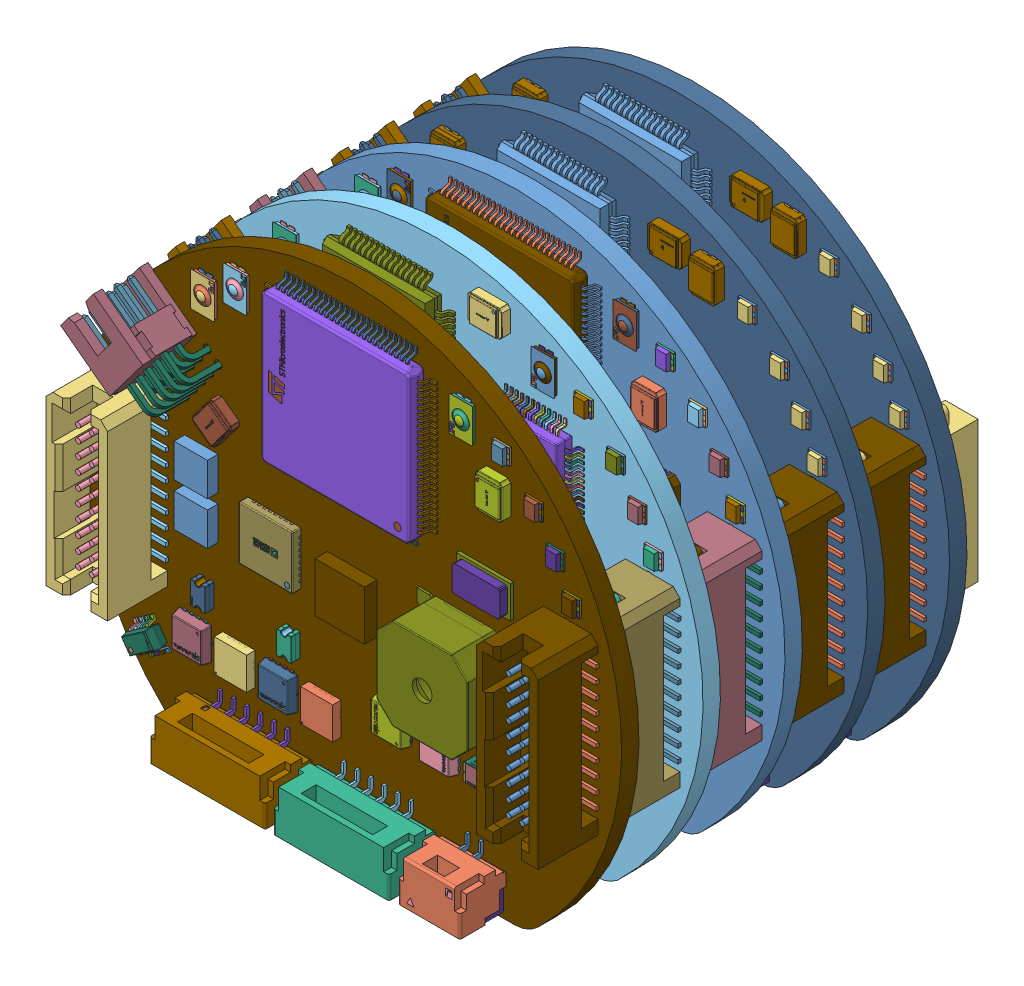
SolidWorks assembly ASSY_HYDRA_MASTER, configuration Default. Lengths in mm.
Overall size (50.15 44.15 42.22).
698 component instances, 436 part files, 12 mates.
Components (placement in the parent):
- HYDRA_V4_NAV-1: HYDRA_V4_NAV [Default] at origin size (50 44 11.77)
  - Open CASCADE STEP translator 7.5 734-1: Open CASCADE STEP translator 7.5 734 [Default] at origin size (50 44 1.75)
  - Open CASCADE STEP translator 7.5 766-1: Open CASCADE STEP translator 7.5 766 [Default] at origin size (2.53 3.23 1.01)
  - Open CASCADE STEP translator 7.5 767-1: Open CASCADE STEP translator 7.5 767 [Default] at origin size (2.5 3.2 0)
  - Open CASCADE STEP translator 7.5 769-1: Open CASCADE STEP translator 7.5 769 [Default] at origin size (0.26 1.24 0)
  - Open CASCADE STEP translator 7.5 770-1: Open CASCADE STEP translator 7.5 770 [Default] at origin size (2.9 1.6 1.31)
  - Open CASCADE STEP translator 7.5 771-1: Open CASCADE STEP translator 7.5 771 [Default] at origin size (0.3 0.6 0.86)
  - Open CASCADE STEP translator 7.5 772-1: Open CASCADE STEP translator 7.5 772 [Default] at origin size (0.3 0.6 0.86)
  - Open CASCADE STEP translator 7.5 773-1: Open CASCADE STEP translator 7.5 773 [Default] at origin size (0.3 0.6 0.86)
  - Open CASCADE STEP translator 7.5 774-1: Open CASCADE STEP translator 7.5 774 [Default] at origin size (0.3 0.6 0.86)
  - Open CASCADE STEP translator 7.5 775-1: Open CASCADE STEP translator 7.5 775 [Default] at origin size (0.4 0.4 0.01)
  - Open CASCADE STEP translator 7.5 776-1: Open CASCADE STEP translator 7.5 776 [Default] at origin size (0.29 1.22 0.01)
  - Open CASCADE STEP translator 7.5 777-1: Open CASCADE STEP translator 7.5 777 [Default] at origin size (0.3 0.6 0.86)
  - Open CASCADE STEP translator 7.5 778-1: Open CASCADE STEP translator 7.5 778 [Default] at origin size (0.3 0.6 0.86)
  - Open CASCADE STEP translator 7.5 779-1: Open CASCADE STEP translator 7.5 779 [Default] at origin size (0.3 0.6 0.86)
  - Open CASCADE STEP translator 7.5 780-1: Open CASCADE STEP translator 7.5 780 [Default] at origin size (0.3 0.6 0.86)
  - Open CASCADE STEP translator 7.5 781-1: Open CASCADE STEP translator 7.5 781 [Default] at origin size (3.25 2.93 1.32)
  - Open CASCADE STEP translator 7.5 782-1: Open CASCADE STEP translator 7.5 782 [Default] at origin size (0.59 0.66 0.86)
  - Open CASCADE STEP translator 7.5 783-1: Open CASCADE STEP translator 7.5 783 [Default] at origin size (0.59 0.66 0.86)
  - Open CASCADE STEP translator 7.5 784-1: Open CASCADE STEP translator 7.5 784 [Default] at origin size (0.59 0.66 0.86)
  - Open CASCADE STEP translator 7.5 785-1: Open CASCADE STEP translator 7.5 785 [Default] at origin size (0.59 0.66 0.86)
  - Open CASCADE STEP translator 7.5 786-1: Open CASCADE STEP translator 7.5 786 [Default] at origin size (0.4 0.4 0.01)
  - Open CASCADE STEP translator 7.5 787-1: Open CASCADE STEP translator 7.5 787 [Default] at origin size (0.65 1.09 0.01)
  - Open CASCADE STEP translator 7.5 788-1: Open CASCADE STEP translator 7.5 788 [Default] at origin size (0.59 0.66 0.86)
  - Open CASCADE STEP translator 7.5 789-1: Open CASCADE STEP translator 7.5 789 [Default] at origin size (0.59 0.66 0.86)
  - Open CASCADE STEP translator 7.5 790-1: Open CASCADE STEP translator 7.5 790 [Default] at origin size (0.59 0.66 0.86)
  - Open CASCADE STEP translator 7.5 791-1: Open CASCADE STEP translator 7.5 791 [Default] at origin size (0.59 0.66 0.86)
  - Open CASCADE STEP translator 7.5 833-1: Open CASCADE STEP translator 7.5 833 [Default] at origin size (0.2 2.2 2.05)
  - Open CASCADE STEP translator 7.5 834-1: Open CASCADE STEP translator 7.5 834 [Default] at origin size (0.2 2.2 2.05)
  - Open CASCADE STEP translator 7.5 835-1: Open CASCADE STEP translator 7.5 835 [Default] at origin size (1.45 1.3 1.05)
  - Open CASCADE STEP translator 7.5 836-1: Open CASCADE STEP translator 7.5 836 [Default] at origin size (5.75 4.05 4.25)
  - Open CASCADE STEP translator 7.5 837-1: Open CASCADE STEP translator 7.5 837 [Default] at origin size (1.45 2.03 0.46)
  - Open CASCADE STEP translator 7.5 838-1: Open CASCADE STEP translator 7.5 838 [Default] at origin size (4.2 3.06 0.01)
  - Open CASCADE STEP translator 7.5 839-1: Open CASCADE STEP translator 7.5 839 [Default] at origin size (14.1 15.2 1.88)
  - Open CASCADE STEP translator 7.5 863-1: Open CASCADE STEP translator 7.5 863 [Default] at origin size (4.1 4.1 0.98)
  - Open CASCADE STEP translator 7.5 864-1: Open CASCADE STEP translator 7.5 864 [Default] at origin size (4.53 6.4 0.96)
  - Open CASCADE STEP translator 7.5 865-1: Open CASCADE STEP translator 7.5 865 [Default] at origin size (6.2 6.4 0.64)
  - Open CASCADE STEP translator 7.5 866-1: Open CASCADE STEP translator 7.5 866 [Default] at origin size (5.96 5.96 2.39)
  - Open CASCADE STEP translator 7.5 867-1: Open CASCADE STEP translator 7.5 867 [Default] at origin size (4.4 4.4 0.72)
  - Open CASCADE STEP translator 7.5 868-1: Open CASCADE STEP translator 7.5 868 [Default] at origin size (6.1 6 0)
  - Open CASCADE STEP translator 7.5 869-1: Open CASCADE STEP translator 7.5 869 [Default] at origin size (0.75 2.66 0)
  - Open CASCADE STEP translator 7.5 870-1: Open CASCADE STEP translator 7.5 870 [Default] at origin size (3.1 3.1 1)
  - Open CASCADE STEP translator 7.5 871-1: Open CASCADE STEP translator 7.5 871 [Default] at origin size (3 2.5 0.81)
  - Open CASCADE STEP translator 7.5 1038-1: Open CASCADE STEP translator 7.5 1038 [Default] at origin size (1.6 1.5 0.2)
  - Open CASCADE STEP translator 7.5 1039-1: Open CASCADE STEP translator 7.5 1039 [Default] at origin size (1.6 1.4 0.19)
  - Open CASCADE STEP translator 7.5 1040-1: Open CASCADE STEP translator 7.5 1040 [Default] at origin size (1.1 1.5 0.36)
  - Open CASCADE STEP translator 7.5 1113-1: Open CASCADE STEP translator 7.5 1113 [Default] at origin size (4.71 4.67 1.1)
  - Open CASCADE STEP translator 7.5 1118-1: Open CASCADE STEP translator 7.5 1118 [Default] at origin size (1.6 1.5 0.2)
  - Open CASCADE STEP translator 7.5 1119-1: Open CASCADE STEP translator 7.5 1119 [Default] at origin size (1.6 1.4 0.19)
  - Open CASCADE STEP translator 7.5 1120-1: Open CASCADE STEP translator 7.5 1120 [Default] at origin size (1.1 1.5 0.36)
  - Open CASCADE STEP translator 7.5 1124-1: Open CASCADE STEP translator 7.5 1124 [Default] at origin size (10.4 9.7 2.7)
  - Open CASCADE STEP translator 7.5 1125-1: Open CASCADE STEP translator 7.5 1125 [Default] at origin size (5 3 0.3)
  - Open CASCADE STEP translator 7.5 1126-1: Open CASCADE STEP translator 7.5 1126 [Default] at origin size (4.46 2.46 0.7)
  - Open CASCADE STEP translator 7.5 1127-1: Open CASCADE STEP translator 7.5 1127 [Default] at origin size (4.6 4.6 1.15)
  - Open CASCADE STEP translator 7.5 1128-1: Open CASCADE STEP translator 7.5 1128 [Default] at origin size (14 14 1.52)
  - Open CASCADE STEP translator 7.5 1129-1: Open CASCADE STEP translator 7.5 1129 [Default] at origin size (16 12.22 0.95)
  - Open CASCADE STEP translator 7.5 1130-1: Open CASCADE STEP translator 7.5 1130 [Default] at origin size (12.22 16 0.95)
  - Open CASCADE STEP translator 7.5 1131-1: Open CASCADE STEP translator 7.5 1131 [Default] at origin size (12.33 12.46 0.1)
  - Open CASCADE STEP translator 7.5 1132-1: Open CASCADE STEP translator 7.5 1132 [Default] at origin size (1.3 3.5 0.06)
  - Open CASCADE STEP translator 7.5 1133-1: Open CASCADE STEP translator 7.5 1133 [Default] at origin size (2 3 0.57)
  - Open CASCADE STEP translator 7.5 1134-1: Open CASCADE STEP translator 7.5 1134 [Default] at origin size (2.2 3.2 0.32)
  - Open CASCADE STEP translator 7.5 1135-1: Open CASCADE STEP translator 7.5 1135 [Default] at origin size (0.46 0.93 0.01)
  - Open CASCADE STEP translator 7.5 1136-1: Open CASCADE STEP translator 7.5 1136 [Default] at origin size (1.3 3.5 0.06)
  - Open CASCADE STEP translator 7.5 1137-1: Open CASCADE STEP translator 7.5 1137 [Default] at origin size (2 3 0.57)
  - Open CASCADE STEP translator 7.5 1138-1: Open CASCADE STEP translator 7.5 1138 [Default] at origin size (2.2 3.2 0.32)
  - Open CASCADE STEP translator 7.5 1139-1: Open CASCADE STEP translator 7.5 1139 [Default] at origin size (0.46 0.93 0.01)
  - Open CASCADE STEP translator 7.5 1209-1: Open CASCADE STEP translator 7.5 1209 [Default] at origin size (2.6 2.6 0.35)
  - Open CASCADE STEP translator 7.5 1210-1: Open CASCADE STEP translator 7.5 1210 [Default] at origin size (7.98 7.97 5.08)
  - Open CASCADE STEP translator 7.5 1211-1: Open CASCADE STEP translator 7.5 1211 [Default] at origin size (6.65 6.86 1.68)
  - Open CASCADE STEP translator 7.5 1212-1: Open CASCADE STEP translator 7.5 1212 [Default] at origin size (6.1 6.49 5.65)
  - Open CASCADE STEP translator 7.5 1213-1: Open CASCADE STEP translator 7.5 1213 [Default] at origin size (11.95 7.6 2.76)
  - Open CASCADE STEP translator 7.5 1214-1: Open CASCADE STEP translator 7.5 1214 [Default] at origin size (1.9 6.7 2.22)
  - Open CASCADE STEP translator 7.5 1215-1: Open CASCADE STEP translator 7.5 1215 [Default] at origin size (6.4 5 1.77)
  - Open CASCADE STEP translator 7.5 1216-1: Open CASCADE STEP translator 7.5 1216 [Default] at origin size (4.77 4.35 0.13)
  - Open CASCADE STEP translator 7.5 1217-1: Open CASCADE STEP translator 7.5 1217 [Default] at origin size (1.9 6.7 2.22)
  - Open CASCADE STEP translator 7.5 1293-1: Open CASCADE STEP translator 7.5 1293 [Default] at origin size (1.6 1.5 0.2)
  - Open CASCADE STEP translator 7.5 1294-1: Open CASCADE STEP translator 7.5 1294 [Default] at origin size (1.6 1.4 0.19)
  - Open CASCADE STEP translator 7.5 1295-1: Open CASCADE STEP translator 7.5 1295 [Default] at origin size (1.1 1.5 0.36)
  - Open CASCADE STEP translator 7.5 1296-1: Open CASCADE STEP translator 7.5 1296 [Default] at origin size (1.6 1.5 0.2)
  - Open CASCADE STEP translator 7.5 1297-1: Open CASCADE STEP translator 7.5 1297 [Default] at origin size (1.6 1.4 0.19)
  - Open CASCADE STEP translator 7.5 1298-1: Open CASCADE STEP translator 7.5 1298 [Default] at origin size (1.1 1.5 0.36)
  - Open CASCADE STEP translator 7.5 1299-1: Open CASCADE STEP translator 7.5 1299 [Default] at origin size (1.3 3.5 0.06)
  - Open CASCADE STEP translator 7.5 1300-1: Open CASCADE STEP translator 7.5 1300 [Default] at origin size (2 3 0.57)
  - Open CASCADE STEP translator 7.5 1301-1: Open CASCADE STEP translator 7.5 1301 [Default] at origin size (2.2 3.2 0.32)
  - Open CASCADE STEP translator 7.5 1302-1: Open CASCADE STEP translator 7.5 1302 [Default] at origin size (0.46 0.93 0.01)
  - Open CASCADE STEP translator 7.5 1303-1: Open CASCADE STEP translator 7.5 1303 [Default] at origin size (5.72 15.88 6.73)
  - Open CASCADE STEP translator 7.5 1304-1: Open CASCADE STEP translator 7.5 1304 [Default] at origin size (1.78 12.7 4.01)
  - Open CASCADE STEP translator 7.5 1305-1: Open CASCADE STEP translator 7.5 1305 [Default] at origin size (5.84 12.7 0.83)
  - Open CASCADE STEP translator 7.5 1306-1: Open CASCADE STEP translator 7.5 1306 [Default] at origin size (5.72 15.88 6.73)
  - Open CASCADE STEP translator 7.5 1307-1: Open CASCADE STEP translator 7.5 1307 [Default] at origin size (1.78 12.7 4.01)
  - Open CASCADE STEP translator 7.5 1308-1: Open CASCADE STEP translator 7.5 1308 [Default] at origin size (5.84 12.7 0.83)
  - Open CASCADE STEP translator 7.5 1309-1: Open CASCADE STEP translator 7.5 1309 [Default] at origin size (3.68 15.88 5.84)
  - Open CASCADE STEP translator 7.5 1310-1: Open CASCADE STEP translator 7.5 1310 [Default] at origin size (4.09 12.7 1.18)
  - Open CASCADE STEP translator 7.5 1311-1: Open CASCADE STEP translator 7.5 1311 [Default] at origin size (3.68 15.88 5.84)
  - Open CASCADE STEP translator 7.5 1312-1: Open CASCADE STEP translator 7.5 1312 [Default] at origin size (4.09 12.7 1.18)
- HYDRA_V4_LINK_V2-1: HYDRA_V4_LINK_V2 [Default] at (-0.0024 -0.0016 7.6116) size (50 44 11.77)
  - Open CASCADE STEP translator 7.5 1-1: Open CASCADE STEP translator 7.5 1 [Default] at origin size (50 44 1.61)
  - Open CASCADE STEP translator 7.5 16-1: Open CASCADE STEP translator 7.5 16 [Default] at origin size (13.25 4.05 4.25)
  - Open CASCADE STEP translator 7.5 17-1: Open CASCADE STEP translator 7.5 17 [Default] at origin size (0.2 4.65 2.09)
  - Open CASCADE STEP translator 7.5 18-1: Open CASCADE STEP translator 7.5 18 [Default] at origin size (0.2 4.65 2.09)
  - Open CASCADE STEP translator 7.5 19-1: Open CASCADE STEP translator 7.5 19 [Default] at origin size (0.2 4.65 2.09)
  - Open CASCADE STEP translator 7.5 20-1: Open CASCADE STEP translator 7.5 20 [Default] at origin size (0.2 4.65 2.09)
  - Open CASCADE STEP translator 7.5 21-1: Open CASCADE STEP translator 7.5 21 [Default] at origin size (0.2 4.65 2.09)
  - Open CASCADE STEP translator 7.5 22-1: Open CASCADE STEP translator 7.5 22 [Default] at origin size (0.2 4.65 2.09)
  - Open CASCADE STEP translator 7.5 23-1: Open CASCADE STEP translator 7.5 23 [Default] at origin size (0.2 4.65 2.09)
  - Open CASCADE STEP translator 7.5 24-1: Open CASCADE STEP translator 7.5 24 [Default] at origin size (0.2 4.65 2.09)
  - Open CASCADE STEP translator 7.5 86-1: Open CASCADE STEP translator 7.5 86 [Default] at origin size (2.15 1.35 0.85)
  - Open CASCADE STEP translator 7.5 87-1: Open CASCADE STEP translator 7.5 87 [Default] at origin size (2.15 1.35 0.85)
  - Open CASCADE STEP translator 7.5 88-1: Open CASCADE STEP translator 7.5 88 [Default] at origin size (1.21 0.73 0.02)
  - Open CASCADE STEP translator 7.5 89-1: Open CASCADE STEP translator 7.5 89 [Default] at origin size (3.23 2.53 1.01)
  - Open CASCADE STEP translator 7.5 90-1: Open CASCADE STEP translator 7.5 90 [Default] at origin size (3.2 2.5 0)
  - Open CASCADE STEP translator 7.5 91-1: Open CASCADE STEP translator 7.5 91 [Default] at origin size (0.25 0.25 0.01)
  - Open CASCADE STEP translator 7.5 92-1: Open CASCADE STEP translator 7.5 92 [Default] at origin size (1.24 0.26 0)
  - Open CASCADE STEP translator 7.5 93-1: Open CASCADE STEP translator 7.5 93 [Default] at origin size (3.25 2.93 1.32)
  - Open CASCADE STEP translator 7.5 94-1: Open CASCADE STEP translator 7.5 94 [Default] at origin size (0.59 0.66 0.86)
  - Open CASCADE STEP translator 7.5 95-1: Open CASCADE STEP translator 7.5 95 [Default] at origin size (0.59 0.66 0.86)
  - Open CASCADE STEP translator 7.5 96-1: Open CASCADE STEP translator 7.5 96 [Default] at origin size (0.59 0.66 0.86)
  - Open CASCADE STEP translator 7.5 97-1: Open CASCADE STEP translator 7.5 97 [Default] at origin size (0.59 0.66 0.86)
  - Open CASCADE STEP translator 7.5 98-1: Open CASCADE STEP translator 7.5 98 [Default] at origin size (0.4 0.4 0.01)
  - Open CASCADE STEP translator 7.5 99-1: Open CASCADE STEP translator 7.5 99 [Default] at origin size (0.65 1.09 0.01)
  - Open CASCADE STEP translator 7.5 100-1: Open CASCADE STEP translator 7.5 100 [Default] at origin size (0.59 0.66 0.86)
  - Open CASCADE STEP translator 7.5 101-1: Open CASCADE STEP translator 7.5 101 [Default] at origin size (0.59 0.66 0.86)
  - Open CASCADE STEP translator 7.5 102-1: Open CASCADE STEP translator 7.5 102 [Default] at origin size (0.59 0.66 0.86)
  - Open CASCADE STEP translator 7.5 103-1: Open CASCADE STEP translator 7.5 103 [Default] at origin size (0.59 0.66 0.86)
  - Open CASCADE STEP translator 7.5 104-1: Open CASCADE STEP translator 7.5 104 [Default] at origin size (4.71 4.67 1.1)
  - Open CASCADE STEP translator 7.5 105-1: Open CASCADE STEP translator 7.5 105 [Default] at origin size (11.99 11.99 1.61)
  - Open CASCADE STEP translator 7.5 106-1: Open CASCADE STEP translator 7.5 106 [Default] at origin size (1.3 3.5 0.06)
  - Open CASCADE STEP translator 7.5 107-1: Open CASCADE STEP translator 7.5 107 [Default] at origin size (2 3 0.57)
  - Open CASCADE STEP translator 7.5 108-1: Open CASCADE STEP translator 7.5 108 [Default] at origin size (2.2 3.2 0.32)
  - Open CASCADE STEP translator 7.5 109-1: Open CASCADE STEP translator 7.5 109 [Default] at origin size (0.46 0.93 0.01)
  - Open CASCADE STEP translator 7.5 157-1: Open CASCADE STEP translator 7.5 157 [Default] at origin size (3.23 2.53 1.01)
  - Open CASCADE STEP translator 7.5 158-1: Open CASCADE STEP translator 7.5 158 [Default] at origin size (3.2 2.5 0)
  - Open CASCADE STEP translator 7.5 159-1: Open CASCADE STEP translator 7.5 159 [Default] at origin size (0.25 0.25 0.01)
  - Open CASCADE STEP translator 7.5 160-1: Open CASCADE STEP translator 7.5 160 [Default] at origin size (1.24 0.26 0)
  - Open CASCADE STEP translator 7.5 161-1: Open CASCADE STEP translator 7.5 161 [Default] at origin size (0.88 0.88 0)
  - Open CASCADE STEP translator 7.5 162-1: Open CASCADE STEP translator 7.5 162 [Default] at origin size (7.01 7.01 1.57)
  - Open CASCADE STEP translator 7.5 163-1: Open CASCADE STEP translator 7.5 163 [Default] at origin size (0.22 1 0.88)
  - Open CASCADE STEP translator 7.5 164-1: Open CASCADE STEP translator 7.5 164 [Default] at origin size (0.22 1 0.88)
  - Open CASCADE STEP translator 7.5 165-1: Open CASCADE STEP translator 7.5 165 [Default] at origin size (0.22 1 0.88)
  - Open CASCADE STEP translator 7.5 166-1: Open CASCADE STEP translator 7.5 166 [Default] at origin size (0.22 1 0.88)
  - Open CASCADE STEP translator 7.5 167-1: Open CASCADE STEP translator 7.5 167 [Default] at origin size (0.22 1 0.88)
  - Open CASCADE STEP translator 7.5 168-1: Open CASCADE STEP translator 7.5 168 [Default] at origin size (0.22 1 0.88)
  - Open CASCADE STEP translator 7.5 169-1: Open CASCADE STEP translator 7.5 169 [Default] at origin size (0.22 1 0.88)
  - Open CASCADE STEP translator 7.5 170-1: Open CASCADE STEP translator 7.5 170 [Default] at origin size (0.22 1 0.88)
  - Open CASCADE STEP translator 7.5 171-1: Open CASCADE STEP translator 7.5 171 [Default] at origin size (0.22 1 0.88)
  - Open CASCADE STEP translator 7.5 172-1: Open CASCADE STEP translator 7.5 172 [Default] at origin size (0.22 1 0.88)
  - Open CASCADE STEP translator 7.5 173-1: Open CASCADE STEP translator 7.5 173 [Default] at origin size (0.22 1 0.88)
  - Open CASCADE STEP translator 7.5 174-1: Open CASCADE STEP translator 7.5 174 [Default] at origin size (0.22 1 0.88)
  - Open CASCADE STEP translator 7.5 175-1: Open CASCADE STEP translator 7.5 175 [Default] at origin size (0.22 1 0.88)
  - Open CASCADE STEP translator 7.5 176-1: Open CASCADE STEP translator 7.5 176 [Default] at origin size (0.22 1 0.88)
  - Open CASCADE STEP translator 7.5 177-1: Open CASCADE STEP translator 7.5 177 [Default] at origin size (0.22 1 0.88)
  - Open CASCADE STEP translator 7.5 178-1: Open CASCADE STEP translator 7.5 178 [Default] at origin size (0.22 1 0.88)
  - Open CASCADE STEP translator 7.5 179-1: Open CASCADE STEP translator 7.5 179 [Default] at origin size (0.22 1 0.88)
  - Open CASCADE STEP translator 7.5 180-1: Open CASCADE STEP translator 7.5 180 [Default] at origin size (0.22 1 0.88)
  - Open CASCADE STEP translator 7.5 181-1: Open CASCADE STEP translator 7.5 181 [Default] at origin size (0.22 1 0.88)
  - Open CASCADE STEP translator 7.5 182-1: Open CASCADE STEP translator 7.5 182 [Default] at origin size (0.22 1 0.88)
  - Open CASCADE STEP translator 7.5 183-1: Open CASCADE STEP translator 7.5 183 [Default] at origin size (0.22 1 0.88)
  - Open CASCADE STEP translator 7.5 184-1: Open CASCADE STEP translator 7.5 184 [Default] at origin size (0.22 1 0.88)
  - Open CASCADE STEP translator 7.5 185-1: Open CASCADE STEP translator 7.5 185 [Default] at origin size (0.22 1 0.88)
  - Open CASCADE STEP translator 7.5 186-1: Open CASCADE STEP translator 7.5 186 [Default] at origin size (0.22 1 0.88)
  - Open CASCADE STEP translator 7.5 187-1: Open CASCADE STEP translator 7.5 187 [Default] at origin size (1 0.22 0.88)
  - Open CASCADE STEP translator 7.5 188-1: Open CASCADE STEP translator 7.5 188 [Default] at origin size (1 0.22 0.88)
  - Open CASCADE STEP translator 7.5 189-1: Open CASCADE STEP translator 7.5 189 [Default] at origin size (1 0.22 0.88)
  - Open CASCADE STEP translator 7.5 190-1: Open CASCADE STEP translator 7.5 190 [Default] at origin size (1 0.22 0.88)
  - Open CASCADE STEP translator 7.5 191-1: Open CASCADE STEP translator 7.5 191 [Default] at origin size (1 0.22 0.88)
  - Open CASCADE STEP translator 7.5 192-1: Open CASCADE STEP translator 7.5 192 [Default] at origin size (1 0.22 0.88)
  - Open CASCADE STEP translator 7.5 193-1: Open CASCADE STEP translator 7.5 193 [Default] at origin size (1 0.22 0.88)
  - Open CASCADE STEP translator 7.5 194-1: Open CASCADE STEP translator 7.5 194 [Default] at origin size (1 0.22 0.88)
  - Open CASCADE STEP translator 7.5 195-1: Open CASCADE STEP translator 7.5 195 [Default] at origin size (1 0.22 0.88)
  - Open CASCADE STEP translator 7.5 196-1: Open CASCADE STEP translator 7.5 196 [Default] at origin size (1 0.22 0.88)
  - Open CASCADE STEP translator 7.5 197-1: Open CASCADE STEP translator 7.5 197 [Default] at origin size (1 0.22 0.88)
  - Open CASCADE STEP translator 7.5 198-1: Open CASCADE STEP translator 7.5 198 [Default] at origin size (1 0.22 0.88)
  - Open CASCADE STEP translator 7.5 199-1: Open CASCADE STEP translator 7.5 199 [Default] at origin size (1 0.22 0.88)
  - Open CASCADE STEP translator 7.5 200-1: Open CASCADE STEP translator 7.5 200 [Default] at origin size (1 0.22 0.88)
  - Open CASCADE STEP translator 7.5 201-1: Open CASCADE STEP translator 7.5 201 [Default] at origin size (1 0.22 0.88)
  - Open CASCADE STEP translator 7.5 202-1: Open CASCADE STEP translator 7.5 202 [Default] at origin size (1 0.22 0.88)
  - Open CASCADE STEP translator 7.5 203-1: Open CASCADE STEP translator 7.5 203 [Default] at origin size (1 0.22 0.88)
  - Open CASCADE STEP translator 7.5 204-1: Open CASCADE STEP translator 7.5 204 [Default] at origin size (1 0.22 0.88)
  - Open CASCADE STEP translator 7.5 205-1: Open CASCADE STEP translator 7.5 205 [Default] at origin size (1 0.22 0.88)
  - Open CASCADE STEP translator 7.5 206-1: Open CASCADE STEP translator 7.5 206 [Default] at origin size (1 0.22 0.88)
  - Open CASCADE STEP translator 7.5 207-1: Open CASCADE STEP translator 7.5 207 [Default] at origin size (1 0.22 0.88)
  - Open CASCADE STEP translator 7.5 208-1: Open CASCADE STEP translator 7.5 208 [Default] at origin size (1 0.22 0.88)
  - Open CASCADE STEP translator 7.5 209-1: Open CASCADE STEP translator 7.5 209 [Default] at origin size (1 0.22 0.88)
  - Open CASCADE STEP translator 7.5 210-1: Open CASCADE STEP translator 7.5 210 [Default] at origin size (1 0.22 0.88)
  - Open CASCADE STEP translator 7.5 212-1: Open CASCADE STEP translator 7.5 212 [Default] at origin size (3 3 1)
  - Open CASCADE STEP translator 7.5 213-1: Open CASCADE STEP translator 7.5 213 [Default] at origin size (3 3 0.8)
  - Open CASCADE STEP translator 7.5 215-1: Open CASCADE STEP translator 7.5 215 [Default] at origin size (4 3 0.2)
  - Open CASCADE STEP translator 7.5 216-1: Open CASCADE STEP translator 7.5 216 [Default] at origin size (4.02 3.02 0.99)
  - Open CASCADE STEP translator 7.5 217-1: Open CASCADE STEP translator 7.5 217 [Default] at origin size (0.36 1.52 0.02)
  - Open CASCADE STEP translator 7.5 218-1: Open CASCADE STEP translator 7.5 218 [Default] at origin size (0.3 0.3 0.01)
  - Open CASCADE STEP translator 7.5 219-1: Open CASCADE STEP translator 7.5 219 [Default] at origin size (3 3 0.8)
  - Open CASCADE STEP translator 7.5 220-1: Open CASCADE STEP translator 7.5 220 [Default] at origin size (2 2 0.8)
  - Open CASCADE STEP translator 7.5 221-1: Open CASCADE STEP translator 7.5 221 [Default] at origin size (3.1 3.1 1)
  - Open CASCADE STEP translator 7.5 222-1: Open CASCADE STEP translator 7.5 222 [Default] at origin size (3.1 3.1 1)
  - Open CASCADE STEP translator 7.5 223-1: Open CASCADE STEP translator 7.5 223 [Default] at origin size (12.71 9.54 2.17)
  - Open CASCADE STEP translator 7.5 509-1: Open CASCADE STEP translator 7.5 509 [Default] at origin size (4.07 4.06 1.2)
  - Open CASCADE STEP translator 7.5 510-1: Open CASCADE STEP translator 7.5 510 [Default] at origin size (2 4.45 0.9)
  - Open CASCADE STEP translator 7.5 511-1: Open CASCADE STEP translator 7.5 511 [Default] at origin size (1.26 1.48 0.01)
  - Open CASCADE STEP translator 7.5 512-1: Open CASCADE STEP translator 7.5 512 [Default] at origin size (3.99 3.99 0.1)
  - Open CASCADE STEP translator 7.5 513-1: Open CASCADE STEP translator 7.5 513 [Default] at origin size (4.06 4.07 1.2)
  - Open CASCADE STEP translator 7.5 514-1: Open CASCADE STEP translator 7.5 514 [Default] at origin size (4.45 2 0.9)
  - Open CASCADE STEP translator 7.5 515-1: Open CASCADE STEP translator 7.5 515 [Default] at origin size (1.48 1.26 0.01)
  - Open CASCADE STEP translator 7.5 516-1: Open CASCADE STEP translator 7.5 516 [Default] at origin size (3.99 3.99 0.1)
  - Open CASCADE STEP translator 7.5 529-1: Open CASCADE STEP translator 7.5 529 [Default] at origin size (1.6 1.5 0.2)
  - Open CASCADE STEP translator 7.5 530-1: Open CASCADE STEP translator 7.5 530 [Default] at origin size (1.6 1.4 0.19)
  - Open CASCADE STEP translator 7.5 531-1: Open CASCADE STEP translator 7.5 531 [Default] at origin size (1.1 1.5 0.36)
  - Open CASCADE STEP translator 7.5 532-1: Open CASCADE STEP translator 7.5 532 [Default] at origin size (1.6 1.5 0.2)
  - Open CASCADE STEP translator 7.5 533-1: Open CASCADE STEP translator 7.5 533 [Default] at origin size (1.6 1.4 0.19)
  - Open CASCADE STEP translator 7.5 534-1: Open CASCADE STEP translator 7.5 534 [Default] at origin size (1.1 1.5 0.36)
  - Open CASCADE STEP translator 7.5 626-1: Open CASCADE STEP translator 7.5 626 [Default] at origin size (2.8 3.3 2)
  - Open CASCADE STEP translator 7.5 627-1: Open CASCADE STEP translator 7.5 627 [Default] at origin size (2.2 0.8 1)
  - Open CASCADE STEP translator 7.5 628-1: Open CASCADE STEP translator 7.5 628 [Default] at origin size (2.2 0.8 1)
  - Open CASCADE STEP translator 7.5 629-1: Open CASCADE STEP translator 7.5 629 [Default] at origin size (2.11 2.66 0.01)
  - Open CASCADE STEP translator 7.5 636-1: Open CASCADE STEP translator 7.5 636 [Default] at origin size (2.01 1.26 1.46)
  - Open CASCADE STEP translator 7.5 637-1: Open CASCADE STEP translator 7.5 637 [Default] at origin size (1 1.25 1.45)
  - Open CASCADE STEP translator 7.5 638-1: Open CASCADE STEP translator 7.5 638 [Default] at origin size (0.67 0.05 0.01)
  - Open CASCADE STEP translator 7.5 639-1: Open CASCADE STEP translator 7.5 639 [Default] at origin size (1.1 1.25 1.45)
  - Open CASCADE STEP translator 7.5 640-1: Open CASCADE STEP translator 7.5 640 [Default] at origin size (0.46 1.26 1.46)
  - Open CASCADE STEP translator 7.5 641-1: Open CASCADE STEP translator 7.5 641 [Default] at origin size (0.46 1.26 1.46)
  - Open CASCADE STEP translator 7.5 642-1: Open CASCADE STEP translator 7.5 642 [Default] at origin size (0.61 0.15 0.01)
  - Open CASCADE STEP translator 7.5 643-1: Open CASCADE STEP translator 7.5 643 [Default] at origin size (1.1 1.25 1.45)
  - Open CASCADE STEP translator 7.5 644-1: Open CASCADE STEP translator 7.5 644 [Default] at origin size (0.46 1.26 1.46)
  - Open CASCADE STEP translator 7.5 645-1: Open CASCADE STEP translator 7.5 645 [Default] at origin size (0.46 1.26 1.46)
  - Open CASCADE STEP translator 7.5 646-1: Open CASCADE STEP translator 7.5 646 [Default] at origin size (0.61 0.15 0.01)
  - Open CASCADE STEP translator 7.5 662-1: Open CASCADE STEP translator 7.5 662 [Default] at origin size (3.3 2.8 2)
  - Open CASCADE STEP translator 7.5 663-1: Open CASCADE STEP translator 7.5 663 [Default] at origin size (0.8 2.2 1)
  - Open CASCADE STEP translator 7.5 664-1: Open CASCADE STEP translator 7.5 664 [Default] at origin size (0.8 2.2 1)
  - Open CASCADE STEP translator 7.5 665-1: Open CASCADE STEP translator 7.5 665 [Default] at origin size (2.66 2.11 0.01)
  - Open CASCADE STEP translator 7.5 669-1: Open CASCADE STEP translator 7.5 669 [Default] at origin size (1.27 2.02 1.42)
  - Open CASCADE STEP translator 7.5 670-1: Open CASCADE STEP translator 7.5 670 [Default] at origin size (1.25 2 1.4)
  - Open CASCADE STEP translator 7.5 671-1: Open CASCADE STEP translator 7.5 671 [Default] at origin size (0.12 0.53 0.1)
  - Open CASCADE STEP translator 7.5 672-1: Open CASCADE STEP translator 7.5 672 [Default] at origin size (1.27 2.02 1.42)
  - Open CASCADE STEP translator 7.5 673-1: Open CASCADE STEP translator 7.5 673 [Default] at origin size (1.25 2 1.4)
  - Open CASCADE STEP translator 7.5 674-1: Open CASCADE STEP translator 7.5 674 [Default] at origin size (0.12 0.53 0.1)
  - Open CASCADE STEP translator 7.5 675-1: Open CASCADE STEP translator 7.5 675 [Default] at origin size (1.27 2.02 1.42)
  - Open CASCADE STEP translator 7.5 676-1: Open CASCADE STEP translator 7.5 676 [Default] at origin size (1.25 2 1.4)
  - Open CASCADE STEP translator 7.5 677-1: Open CASCADE STEP translator 7.5 677 [Default] at origin size (0.12 0.53 0.1)
  - Open CASCADE STEP translator 7.5 678-1: Open CASCADE STEP translator 7.5 678 [Default] at origin size (1.25 0.5 1.4)
  - Open CASCADE STEP translator 7.5 679-1: Open CASCADE STEP translator 7.5 679 [Default] at origin size (1.25 0.5 1.4)
  - Open CASCADE STEP translator 7.5 680-1: Open CASCADE STEP translator 7.5 680 [Default] at origin size (1.15 1 1.3)
  - Open CASCADE STEP translator 7.5 681-1: Open CASCADE STEP translator 7.5 681 [Default] at origin size (1.25 0.5 1.4)
  - Open CASCADE STEP translator 7.5 682-1: Open CASCADE STEP translator 7.5 682 [Default] at origin size (1.25 0.5 1.4)
  - Open CASCADE STEP translator 7.5 683-1: Open CASCADE STEP translator 7.5 683 [Default] at origin size (1.15 1 1.3)
  - Open CASCADE STEP translator 7.5 687-1: Open CASCADE STEP translator 7.5 687 [Default] at origin size (0.5 1.25 1.4)
  - Open CASCADE STEP translator 7.5 688-1: Open CASCADE STEP translator 7.5 688 [Default] at origin size (0.5 1.25 1.4)
  - Open CASCADE STEP translator 7.5 689-1: Open CASCADE STEP translator 7.5 689 [Default] at origin size (1 1.15 1.3)
  - Open CASCADE STEP translator 7.5 708-1: Open CASCADE STEP translator 7.5 708 [Default] at origin size (1.6 1.5 0.2)
  - Open CASCADE STEP translator 7.5 709-1: Open CASCADE STEP translator 7.5 709 [Default] at origin size (1.6 1.4 0.19)
  - Open CASCADE STEP translator 7.5 710-1: Open CASCADE STEP translator 7.5 710 [Default] at origin size (1.1 1.5 0.36)
  - Open CASCADE STEP translator 7.5 711-1: Open CASCADE STEP translator 7.5 711 [Default] at origin size (1.6 1.5 0.2)
  - Open CASCADE STEP translator 7.5 712-1: Open CASCADE STEP translator 7.5 712 [Default] at origin size (1.6 1.4 0.19)
  - Open CASCADE STEP translator 7.5 713-1: Open CASCADE STEP translator 7.5 713 [Default] at origin size (1.1 1.5 0.36)
  - Open CASCADE STEP translator 7.5 714-1: Open CASCADE STEP translator 7.5 714 [Default] at origin size (17 16 3.32)
  - Open CASCADE STEP translator 7.5 715-1: Open CASCADE STEP translator 7.5 715 [Default] at origin size (3.68 15.88 5.84)
  - Open CASCADE STEP translator 7.5 716-1: Open CASCADE STEP translator 7.5 716 [Default] at origin size (4.09 12.7 1.18)
  - Open CASCADE STEP translator 7.5 717-1: Open CASCADE STEP translator 7.5 717 [Default] at origin size (3.68 15.88 5.84)
  - Open CASCADE STEP translator 7.5 718-1: Open CASCADE STEP translator 7.5 718 [Default] at origin size (4.09 12.7 1.18)
  - Open CASCADE STEP translator 7.5 719-1: Open CASCADE STEP translator 7.5 719 [Default] at origin size (1.3 3.5 0.06)
  - Open CASCADE STEP translator 7.5 720-1: Open CASCADE STEP translator 7.5 720 [Default] at origin size (2 3 0.57)
  - Open CASCADE STEP translator 7.5 721-1: Open CASCADE STEP translator 7.5 721 [Default] at origin size (2.2 3.2 0.32)
  - Open CASCADE STEP translator 7.5 722-1: Open CASCADE STEP translator 7.5 722 [Default] at origin size (0.46 0.93 0.01)
  - Open CASCADE STEP translator 7.5 723-1: Open CASCADE STEP translator 7.5 723 [Default] at origin size (14.1 15.2 1.88)
  - Open CASCADE STEP translator 7.5 725-1: Open CASCADE STEP translator 7.5 725 [Default] at origin size (7.98 7.97 5.08)
  - Open CASCADE STEP translator 7.5 726-1: Open CASCADE STEP translator 7.5 726 [Default] at origin size (6.65 6.86 1.68)
  - Open CASCADE STEP translator 7.5 727-1: Open CASCADE STEP translator 7.5 727 [Default] at origin size (6.1 6.49 5.65)
  - Open CASCADE STEP translator 7.5 728-1: Open CASCADE STEP translator 7.5 728 [Default] at origin size (5.72 15.88 6.73)
  - Open CASCADE STEP translator 7.5 729-1: Open CASCADE STEP translator 7.5 729 [Default] at origin size (1.78 12.7 4.01)
  - Open CASCADE STEP translator 7.5 730-1: Open CASCADE STEP translator 7.5 730 [Default] at origin size (5.84 12.7 0.83)
  - Open CASCADE STEP translator 7.5 731-1: Open CASCADE STEP translator 7.5 731 [Default] at origin size (5.72 15.88 6.73)
  - Open CASCADE STEP translator 7.5 732-1: Open CASCADE STEP translator 7.5 732 [Default] at origin size (1.78 12.7 4.01)
  - Open CASCADE STEP translator 7.5 733-1: Open CASCADE STEP translator 7.5 733 [Default] at origin size (5.84 12.7 0.83)
- HYDRA_V4_RECOVERY-1: HYDRA_V4_RECOVERY [Default] at (-0.0049 -0.0019 15.2232) size (50.1 44.1 11.77)
  - Open CASCADE STEP translator 7.5 2755-1: Open CASCADE STEP translator 7.5 2755 [Default] at origin size (50.1 44.1 1.61)
  - Open CASCADE STEP translator 7.5 2760-1: Open CASCADE STEP translator 7.5 2760 [Default] at origin size (3.1 3.1 1)
  - Open CASCADE STEP translator 7.5 2790-1: Open CASCADE STEP translator 7.5 2790 [Default] at origin size (14.6 14.5 1.9)
  - Open CASCADE STEP translator 7.5 2825-1: Open CASCADE STEP translator 7.5 2825 [Default] at origin size (1.3 3.5 0.06)
  - Open CASCADE STEP translator 7.5 2826-1: Open CASCADE STEP translator 7.5 2826 [Default] at origin size (2 3 0.57)
  - Open CASCADE STEP translator 7.5 2827-1: Open CASCADE STEP translator 7.5 2827 [Default] at origin size (2.2 3.2 0.32)
  - Open CASCADE STEP translator 7.5 2828-1: Open CASCADE STEP translator 7.5 2828 [Default] at origin size (0.46 0.93 0.01)
  - Open CASCADE STEP translator 7.5 2844-1: Open CASCADE STEP translator 7.5 2844 [Default] at origin size (2.53 3.23 1.01)
  - Open CASCADE STEP translator 7.5 2845-1: Open CASCADE STEP translator 7.5 2845 [Default] at origin size (2.5 3.2 0)
  - Open CASCADE STEP translator 7.5 2846-1: Open CASCADE STEP translator 7.5 2846 [Default] at origin size (0.25 0.25 0.01)
  - Open CASCADE STEP translator 7.5 2847-1: Open CASCADE STEP translator 7.5 2847 [Default] at origin size (0.26 1.24 0)
  - Open CASCADE STEP translator 7.5 2848-1: Open CASCADE STEP translator 7.5 2848 [Default] at origin size (3.62 3.76 1.01)
  - Open CASCADE STEP translator 7.5 2849-1: Open CASCADE STEP translator 7.5 2849 [Default] at origin size (3.62 3.76 0)
  - Open CASCADE STEP translator 7.5 2851-1: Open CASCADE STEP translator 7.5 2851 [Default] at origin size (0.81 1.11 0)
  - Open CASCADE STEP translator 7.5 2852-1: Open CASCADE STEP translator 7.5 2852 [Default] at origin size (4.71 4.67 1.1)
  - Open CASCADE STEP translator 7.5 2853-1: Open CASCADE STEP translator 7.5 2853 [Default] at origin size (3.25 2.93 1.32)
  - Open CASCADE STEP translator 7.5 2854-1: Open CASCADE STEP translator 7.5 2854 [Default] at origin size (0.59 0.66 0.86)
  - Open CASCADE STEP translator 7.5 2855-1: Open CASCADE STEP translator 7.5 2855 [Default] at origin size (0.59 0.66 0.86)
  - Open CASCADE STEP translator 7.5 2856-1: Open CASCADE STEP translator 7.5 2856 [Default] at origin size (0.59 0.66 0.86)
  - Open CASCADE STEP translator 7.5 2857-1: Open CASCADE STEP translator 7.5 2857 [Default] at origin size (0.59 0.66 0.86)
  - Open CASCADE STEP translator 7.5 2858-1: Open CASCADE STEP translator 7.5 2858 [Default] at origin size (0.4 0.4 0.01)
  - Open CASCADE STEP translator 7.5 2859-1: Open CASCADE STEP translator 7.5 2859 [Default] at origin size (0.65 1.09 0.01)
  - Open CASCADE STEP translator 7.5 2860-1: Open CASCADE STEP translator 7.5 2860 [Default] at origin size (0.59 0.66 0.86)
  - Open CASCADE STEP translator 7.5 2861-1: Open CASCADE STEP translator 7.5 2861 [Default] at origin size (0.59 0.66 0.86)
  - Open CASCADE STEP translator 7.5 2862-1: Open CASCADE STEP translator 7.5 2862 [Default] at origin size (0.59 0.66 0.86)
  - Open CASCADE STEP translator 7.5 2863-1: Open CASCADE STEP translator 7.5 2863 [Default] at origin size (0.59 0.66 0.86)
  - Open CASCADE STEP translator 7.5 2864-1: Open CASCADE STEP translator 7.5 2864 [Default] at origin size (14 14 1.52)
  - Open CASCADE STEP translator 7.5 2865-1: Open CASCADE STEP translator 7.5 2865 [Default] at origin size (16 12.22 0.95)
  - Open CASCADE STEP translator 7.5 2866-1: Open CASCADE STEP translator 7.5 2866 [Default] at origin size (12.22 16 0.95)
  - Open CASCADE STEP translator 7.5 2867-1: Open CASCADE STEP translator 7.5 2867 [Default] at origin size (12.33 12.46 0.1)
  - Open CASCADE STEP translator 7.5 2868-1: Open CASCADE STEP translator 7.5 2868 [Default] at origin size (5.02 5.02 0.79)
  - Open CASCADE STEP translator 7.5 2869-1: Open CASCADE STEP translator 7.5 2869 [Default] at origin size (5 5 0.2)
  - Open CASCADE STEP translator 7.5 2870-1: Open CASCADE STEP translator 7.5 2870 [Default] at origin size (0.51 0.51 0.01)
  - Open CASCADE STEP translator 7.5 2871-1: Open CASCADE STEP translator 7.5 2871 [Default] at origin size (2.27 0.67 0.03)
  - Open CASCADE STEP translator 7.5 2873-1: Open CASCADE STEP translator 7.5 2873 [Default] at origin size (5 3 0.3)
  - Open CASCADE STEP translator 7.5 2874-1: Open CASCADE STEP translator 7.5 2874 [Default] at origin size (4.46 2.46 0.7)
  - Open CASCADE STEP translator 7.5 2875-1: Open CASCADE STEP translator 7.5 2875 [Default] at origin size (4.6 4.6 1.15)
  - Open CASCADE STEP translator 7.5 2876-1: Open CASCADE STEP translator 7.5 2876 [Default] at origin size (3.1 3.1 1)
  - Open CASCADE STEP translator 7.5 2877-1: Open CASCADE STEP translator 7.5 2877 [Default] at origin size (3 3 0.8)
  - Open CASCADE STEP translator 7.5 2878-1: Open CASCADE STEP translator 7.5 2878 [Default] at origin size (3 3 0.8)
  - Open CASCADE STEP translator 7.5 3138-1: Open CASCADE STEP translator 7.5 3138 [Default] at origin size (3 3 0.86)
  - Open CASCADE STEP translator 7.5 3139-1: Open CASCADE STEP translator 7.5 3139 [Default] at origin size (3.2 3.1 0.15)
  - Open CASCADE STEP translator 7.5 3140-1: Open CASCADE STEP translator 7.5 3140 [Default] at origin size (0.53 2.36 0.02)
  - Open CASCADE STEP translator 7.5 3141-1: Open CASCADE STEP translator 7.5 3141 [Default] at origin size (3 3 0.86)
  - Open CASCADE STEP translator 7.5 3142-1: Open CASCADE STEP translator 7.5 3142 [Default] at origin size (3.2 3.1 0.15)
  - Open CASCADE STEP translator 7.5 3143-1: Open CASCADE STEP translator 7.5 3143 [Default] at origin size (0.53 2.36 0.02)
  - Open CASCADE STEP translator 7.5 3148-1: Open CASCADE STEP translator 7.5 3148 [Default] at origin size (3 3 0.86)
  - Open CASCADE STEP translator 7.5 3149-1: Open CASCADE STEP translator 7.5 3149 [Default] at origin size (3.1 3.2 0.15)
  - Open CASCADE STEP translator 7.5 3150-1: Open CASCADE STEP translator 7.5 3150 [Default] at origin size (2.36 0.53 0.02)
  - Open CASCADE STEP translator 7.5 3160-1: Open CASCADE STEP translator 7.5 3160 [Default] at origin size (3 3 0.86)
  - Open CASCADE STEP translator 7.5 3161-1: Open CASCADE STEP translator 7.5 3161 [Default] at origin size (3.1 3.2 0.15)
  - Open CASCADE STEP translator 7.5 3162-1: Open CASCADE STEP translator 7.5 3162 [Default] at origin size (2.36 0.53 0.02)
  - Open CASCADE STEP translator 7.5 3163-1: Open CASCADE STEP translator 7.5 3163 [Default] at origin size (8.53 8.53 4)
  - Open CASCADE STEP translator 7.5 3164-1: Open CASCADE STEP translator 7.5 3164 [Default] at origin size (0.2 2.2 2.05)
  - Open CASCADE STEP translator 7.5 3165-1: Open CASCADE STEP translator 7.5 3165 [Default] at origin size (0.2 2.2 2.05)
  - Open CASCADE STEP translator 7.5 3166-1: Open CASCADE STEP translator 7.5 3166 [Default] at origin size (1.45 1.3 1.05)
  - Open CASCADE STEP translator 7.5 3167-1: Open CASCADE STEP translator 7.5 3167 [Default] at origin size (5.75 4.05 4.25)
  - Open CASCADE STEP translator 7.5 3168-1: Open CASCADE STEP translator 7.5 3168 [Default] at origin size (1.45 2.03 0.46)
  - Open CASCADE STEP translator 7.5 3169-1: Open CASCADE STEP translator 7.5 3169 [Default] at origin size (4.2 3.06 0.01)
  - Open CASCADE STEP translator 7.5 3170-1: Open CASCADE STEP translator 7.5 3170 [Default] at origin size (6.45 4.3 2.13)
  - Open CASCADE STEP translator 7.5 3171-1: Open CASCADE STEP translator 7.5 3171 [Default] at origin size (10.75 4.05 4.35)
  - Open CASCADE STEP translator 7.5 3172-1: Open CASCADE STEP translator 7.5 3172 [Default] at origin size (10.15 2.2 3)
  - Open CASCADE STEP translator 7.5 3174-1: Open CASCADE STEP translator 7.5 3174 [Default] at origin size (6.45 4.3 2.13)
  - Open CASCADE STEP translator 7.5 3175-1: Open CASCADE STEP translator 7.5 3175 [Default] at origin size (10.75 4.05 4.35)
  - Open CASCADE STEP translator 7.5 3176-1: Open CASCADE STEP translator 7.5 3176 [Default] at origin size (10.15 2.2 3)
  - Open CASCADE STEP translator 7.5 3177-1: Open CASCADE STEP translator 7.5 3177 [Default] at origin size (0.46 0.01 0.54)
  - Open CASCADE STEP translator 7.5 3181-1: Open CASCADE STEP translator 7.5 3181 [Default] at origin size (3.2 1.6 1.1)
  - Open CASCADE STEP translator 7.5 3182-1: Open CASCADE STEP translator 7.5 3182 [Default] at origin size (2.7 1.6 0.03)
  - Open CASCADE STEP translator 7.5 3183-1: Open CASCADE STEP translator 7.5 3183 [Default] at origin size (2.7 1.6 0.03)
  - Open CASCADE STEP translator 7.5 3184-1: Open CASCADE STEP translator 7.5 3184 [Default] at origin size (3.2 0.6 1.04)
  - Open CASCADE STEP translator 7.5 3185-1: Open CASCADE STEP translator 7.5 3185 [Default] at origin size (3.2 0.6 1.04)
  - Open CASCADE STEP translator 7.5 3186-1: Open CASCADE STEP translator 7.5 3186 [Default] at origin size (2.2 1.6 0.1)
  - Open CASCADE STEP translator 7.5 3187-1: Open CASCADE STEP translator 7.5 3187 [Default] at origin size (2.2 1.6 0.1)
  - Open CASCADE STEP translator 7.5 3188-1: Open CASCADE STEP translator 7.5 3188 [Default] at origin size (2.2 1.6 0.1)
  - Open CASCADE STEP translator 7.5 3189-1: Open CASCADE STEP translator 7.5 3189 [Default] at origin size (1.21 0.16 0.02)
  - Open CASCADE STEP translator 7.5 3201-1: Open CASCADE STEP translator 7.5 3201 [Default] at origin size (1.35 0.95 0.01)
  - Open CASCADE STEP translator 7.5 3202-1: Open CASCADE STEP translator 7.5 3202 [Default] at origin size (1.35 2.15 0.01)
  - Open CASCADE STEP translator 7.5 3203-1: Open CASCADE STEP translator 7.5 3203 [Default] at origin size (0.65 2.16 0.85)
  - Open CASCADE STEP translator 7.5 3204-1: Open CASCADE STEP translator 7.5 3204 [Default] at origin size (1.35 2.15 0.85)
  - Open CASCADE STEP translator 7.5 3206-1: Open CASCADE STEP translator 7.5 3206 [Default] at origin size (1.35 0.95 0.01)
  - Open CASCADE STEP translator 7.5 3207-1: Open CASCADE STEP translator 7.5 3207 [Default] at origin size (1.35 2.15 0.01)
  - Open CASCADE STEP translator 7.5 3208-1: Open CASCADE STEP translator 7.5 3208 [Default] at origin size (0.65 2.16 0.85)
  - Open CASCADE STEP translator 7.5 3209-1: Open CASCADE STEP translator 7.5 3209 [Default] at origin size (1.35 2.15 0.85)
  - Open CASCADE STEP translator 7.5 3210-1: Open CASCADE STEP translator 7.5 3210 [Default] at origin size (0.09 0.66 0.02)
  - Open CASCADE STEP translator 7.5 3212-1: Open CASCADE STEP translator 7.5 3212 [Default] at origin size (4.32 2.6 2.15)
  - Open CASCADE STEP translator 7.5 3372-1: Open CASCADE STEP translator 7.5 3372 [Default] at origin size (7.98 7.97 5.08)
  - Open CASCADE STEP translator 7.5 3373-1: Open CASCADE STEP translator 7.5 3373 [Default] at origin size (6.65 6.86 1.68)
  - Open CASCADE STEP translator 7.5 3374-1: Open CASCADE STEP translator 7.5 3374 [Default] at origin size (6.1 6.49 5.65)
  - Open CASCADE STEP translator 7.5 3375-1: Open CASCADE STEP translator 7.5 3375 [Default] at origin size (1.6 1.5 0.2)
  - Open CASCADE STEP translator 7.5 3376-1: Open CASCADE STEP translator 7.5 3376 [Default] at origin size (1.6 1.4 0.19)
  - Open CASCADE STEP translator 7.5 3377-1: Open CASCADE STEP translator 7.5 3377 [Default] at origin size (1.1 1.5 0.36)
  - Open CASCADE STEP translator 7.5 3378-1: Open CASCADE STEP translator 7.5 3378 [Default] at origin size (1.3 3.5 0.06)
  - Open CASCADE STEP translator 7.5 3379-1: Open CASCADE STEP translator 7.5 3379 [Default] at origin size (2 3 0.57)
  - Open CASCADE STEP translator 7.5 3380-1: Open CASCADE STEP translator 7.5 3380 [Default] at origin size (2.2 3.2 0.32)
  - Open CASCADE STEP translator 7.5 3381-1: Open CASCADE STEP translator 7.5 3381 [Default] at origin size (0.46 0.93 0.01)
  - Open CASCADE STEP translator 7.5 3382-1: Open CASCADE STEP translator 7.5 3382 [Default] at origin size (1.3 3.5 0.06)
